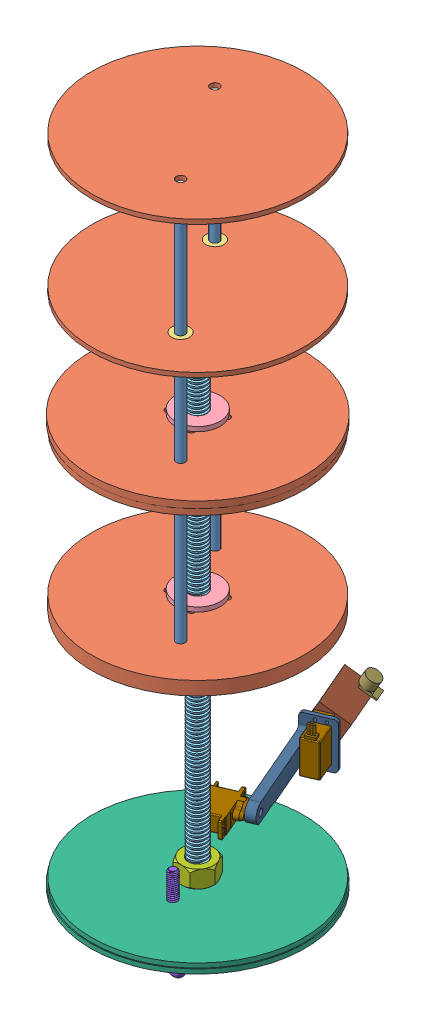
SolidWorks assembly Payload, configuration Default. Lengths in mm.
Overall size (210.78 503.44 275.7).
24 component instances, 15 part files, 42 mates.
Components (placement in the parent):
- Payload Bay-1: Payload Bay [Default] at (141.5956 144.8149 195.4526) size (155.24 279.4 155.24) (hidden)
- Payload Airframe-1: Payload Airframe [Default] at (141.5956 195.6149 195.4526) x (-0.336591 0 -0.941651) z (0.941651 0 -0.336591) size (155.24 254 155.24) (hidden)
- Nosecone-1: Nosecone [Default] at (141.5956 1055.8458 195.4526) x (0 -1 0) z (-0.561903 0 0.827203) size (742.76 155.24 155.24) (hidden)
- Steel Rod-1: Steel Rod [Default] at (119.1458 155.9274 160.8169) x (-0.543909 0 -0.839144) z (0.839144 0 -0.543909) size (6.35 288.93 6.35)
- Steel Rod-2: Steel Rod [Default] at (164.0455 155.9274 230.0882) x (-0.543909 0 -0.839144) z (0.839144 0 -0.543909) size (6.35 288.93 6.35)
- Central Mount-3: Central Mount [Motor Mount] at (141.5956 352.0501 195.4526) x (-0.543909 0 -0.839144) z (0.839144 0 -0.543909) size (150.98 3.17 150.98)
- 6389K627_Light Duty Dry-Running Nylon Sleeve Bearing-1: 6389K627_Light Duty Dry-Running Nylon Sleeve Bearing [6389K627] at (119.1458 355.2251 160.8169) x (0.493731 0 0.869615) z (0.869615 0 -0.493731) size (12.7 9.53 12.7)
- 6389K627_Light Duty Dry-Running Nylon Sleeve Bearing-2: 6389K627_Light Duty Dry-Running Nylon Sleeve Bearing [6389K627] at (164.0455 355.2251 230.0882) x (-0.837169 0 -0.546944) z (-0.546944 0 0.837169) size (12.7 9.53 12.7)
- Central Mount-4: Central Mount [Screw Mount Top] at (141.5956 276.5774 195.4526) x (-0.543909 0 -0.839144) z (-0.839144 0 0.543909) size (152.4 9.53 152.4)
- Central Mount-5: Central Mount [Copy of Screw Mount Bottom] at (141.5956 155.9274 195.4526) x (-0.543909 0 -0.839144) z (0.839144 0 -0.543909) size (150.98 9.53 150.98)
- Central Mount-6: Central Mount [Top Plate] at (141.5956 449.6149 195.4526) x (-0.543909 0 -0.839144) z (-0.839144 0 0.543909) size (150.98 3.17 150.98)
- 95120A111_932 Bearing Bronze Acme Flange Nut-1: 95120A111_932 Bearing Bronze Acme Flange Nut [95120A111] at (141.5956 279.7524 195.4526) x (0.056164 0 0.998422) z (0.998422 0 -0.056164) size (31.75 26.14 31.75)
- 95120A111_932 Bearing Bronze Acme Flange Nut-2: 95120A111_932 Bearing Bronze Acme Flange Nut [95120A111] at (141.5956 168.6274 195.4526) x (0.056164 0 0.998422) z (0.998422 0 -0.056164) size (31.75 26.14 31.75)
- 98935A911_Carbon Steel Acme Lead Screw-1: 98935A911_Carbon Steel Acme Lead Screw [98935A911] at (141.5956 47.2501 195.4526) x (0 1 0) z (-0.83707 0 0.547095) size (382.87 12.7 14.66)
- Bulkhead-1: Bulkhead [Default] at (141.5956 -14.9303 195.4526) x (0.918474 0 -0.395481) z (0.395481 0 0.918474) size (152.4 6.35 152.4)
- 94815A107_Carbon Steel Acme Hex Nut-1: 94815A107_Carbon Steel Acme Hex Nut [94815A107] at (141.5956 -21.0818 195.4526) x (0.073978 0 0.99726) z (0 1 0) size (22.23 28.23 12.35)
- 94815A107_Carbon Steel Acme Hex Nut-2: 94815A107_Carbon Steel Acme Hex Nut [94815A107] at (141.5956 -2.4287 195.4526) x (0.837169 0 0.546944) z (0 1 0) size (22.23 28.23 12.35)
- 3014T45_Steel Eyebolt with Shoulder - for Lifting-1: 3014T45_Steel Eyebolt with Shoulder - for Lifting [3014T45] at (147.1643 -38.7428 218.6369) x (-0.930118 0 -0.367262) z (-0.367262 0 0.930118) size (30.16 64.79 14.29)
- Gimbal Assem-1: Gimbal Assem [Default] at (112.6369 -2.8653 153.4838) x (0 -1 0) z (0.395481 0 0.918474) size (36.8 57.45 135.7) (flexible)
  - Hitec HS-65mg+ Micro Servo v01-1: Hitec HS-65mg+ Micro Servo v01 [Default] at origin size (11.43 28.88 36.23)
  - Camera Arm-1: Camera Arm [Default] at (0 18.675 -37.6301) size (32.79 21.59 76.2)
  - Hitec HS-65mg+ Micro Servo v01-2: Hitec HS-65mg+ Micro Servo v01 [Default] at (0 27.565 -68.0533) x (0 -1 0) z (1 0 0) size (11.43 28.88 36.23)
  - Camera Mount-1: Camera Mount [Default] at (-10.3181 30.0369 -83.5533) x (0.486593 0.873629 0) z (-0.873629 0.486593 0) size (20 35 12.7)
  - Arducam Camera-1: Arducam Camera [Default] at (-8.7661 38.0435 -114.3033) x (-0.486593 -0.873629 0) z (0 0 -1) size (13.5 9 10)
Mates (geometry in assembly coordinates):
- Concentric1: concentric aligned: circle of Payload Bay-1; circle of Payload Airframe-1
- Coincident2: coincident anti-aligned: plane of Payload Bay-1 through (141.5956 195.6149 195.4526) normal (0 1 0); plane of Payload Airframe-1 through (141.5956 195.6149 195.4526) normal (0 -1 0)
- Concentric3: concentric anti-aligned: cylinder of Payload Airframe-1 through (141.5956 449.6149 195.4526) axis (0 -1 0) radius 76.2; cylinder of Nosecone-1 through (141.5956 1055.8458 195.4526) axis (0 1 0) radius 76.2
- Coincident4: coincident anti-aligned: plane of Payload Airframe-1 through (141.5956 449.6149 195.4526) normal (0 1 0); plane of Nosecone-1 through (141.5956 449.6149 195.4526) normal (0 -1 0)
- Concentric6: concentric aligned: circle of Steel Rod-1; cylinder of Central Mount-3 through (119.1458 324.7451 160.8169) axis (0 1 0) radius 4.7625
- Concentric7: concentric anti-aligned: circle of Steel Rod-2; circle of Central Mount-3
- Concentric8: concentric anti-aligned: cylinder of Steel Rod-1 through (119.1458 444.8524 160.8169) axis (0 -1 0) radius 3.175; cylinder of 6389K627_Light Duty Dry-Running Nylon Sleeve Bearing-1 through (119.1458 345.7001 160.8169) axis (0 1 0) radius 3.175
- Coincident10: coincident anti-aligned: plane of Central Mount-3 through (119.1458 353.6376 160.8169) normal (0 1 0); plane of 6389K627_Light Duty Dry-Running Nylon Sleeve Bearing-1 through (119.1458 353.6376 160.8169) normal (0 -1 0)
- Concentric9: concentric anti-aligned: cylinder of Steel Rod-2 through (164.0455 444.8524 230.0882) axis (0 -1 0) radius 3.175; cylinder of 6389K627_Light Duty Dry-Running Nylon Sleeve Bearing-2 through (164.0455 345.7001 230.0882) axis (0 1 0) radius 4.7625
- Coincident11: coincident anti-aligned: plane of Central Mount-3 through (164.0455 353.6376 230.0882) normal (0 1 0); plane of 6389K627_Light Duty Dry-Running Nylon Sleeve Bearing-2 through (164.0455 353.6376 230.0882) normal (0 -1 0)
- Concentric10: concentric aligned: cylinder of Steel Rod-2 through (164.0455 444.8524 230.0882) axis (0 -1 0) radius 3.175; cylinder of Central Mount-4 through (164.0455 276.5774 230.0882) axis (0 -1 0) radius 3.175
- Coincident12: coincident aligned: cylinder of Steel Rod-1 through (119.1458 444.8524 160.8169) axis (0 -1 0) radius 3.175; circle of Central Mount-4
- Concentric11: concentric anti-aligned: cylinder of Steel Rod-2 through (164.0455 444.8524 230.0882) axis (0 -1 0) radius 3.175; cylinder of Central Mount-5 through (164.0455 160.6899 230.0882) axis (0 1 0) radius 3.175
- Concentric12: concentric anti-aligned: cylinder of Payload Bay-1 through (141.5956 -7.5851 195.4526) axis (0 1 0) radius 75.4888; cylinder of Central Mount-5 through (141.5956 165.4524 195.4526) axis (0 -1 0) radius 75.4888
- Coincident15: coincident anti-aligned: plane of Payload Bay-1 through (141.5956 271.8149 195.4526) normal (0 1 0); plane of Central Mount-4 through (141.5956 271.8149 195.4526) normal (0 -1 0)
- Distance1: distance = 101.6 mm anti-aligned: plane of Central Mount-4 through (141.5956 267.0524 195.4526) normal (0 -1 0); plane of Central Mount-5 through (141.5956 165.4524 195.4526) normal (0 1 0)
- Concentric13: concentric aligned: cylinder of Steel Rod-1 through (119.1458 444.8524 160.8169) axis (0 -1 0) radius 3.175; cylinder of Central Mount-6 through (119.1458 451.2024 160.8169) axis (0 -1 0) radius 3.175
- Concentric14: concentric aligned: cylinder of Steel Rod-2 through (164.0455 444.8524 230.0882) axis (0 -1 0) radius 3.175; cylinder of Central Mount-6 through (164.0455 451.2024 230.0882) axis (0 -1 0) radius 3.175
- Coincident17: coincident anti-aligned: circle of Steel Rod-1; circle of Central Mount-6
- Concentric15: concentric aligned: cylinder of Payload Bay-1 through (141.5956 -7.5851 195.4526) axis (0 1 0) radius 76.2; cylinder of Central Mount-4 through (141.5956 267.0524 195.4526) axis (0 1 0) radius 76.2
- Concentric17: concentric aligned: cylinder of Central Mount-4 through (141.5956 305.9144 195.4526) axis (0 -1 0) radius 9.525; cylinder of 95120A111_932 Bearing Bronze Acme Flange Nut-1 through (141.5956 325.1027 195.4526) axis (0 -1 0) radius 9.525
- Coincident19: coincident anti-aligned: plane of Central Mount-4 through (141.5956 276.5774 195.4526) normal (0 1 0); plane of 95120A111_932 Bearing Bronze Acme Flange Nut-1 through (141.5956 276.5774 195.4526) normal (0 -1 0)
- Concentric18: concentric anti-aligned: cylinder of Central Mount-5 through (141.5956 126.5904 195.4526) axis (0 1 0) radius 9.525; cylinder of 95120A111_932 Bearing Bronze Acme Flange Nut-2 through (141.5956 213.9777 195.4526) axis (0 -1 0) radius 9.525
- Coincident20: coincident anti-aligned: plane of Central Mount-5 through (141.5956 165.4524 195.4526) normal (0 1 0); plane of 95120A111_932 Bearing Bronze Acme Flange Nut-2 through (141.5956 165.4524 195.4526) normal (0 -1 0)
- Concentric19: concentric anti-aligned: circle of 95120A111_932 Bearing Bronze Acme Flange Nut-1; circle of 98935A911_Carbon Steel Acme Lead Screw-1
- Coincident21: coincident anti-aligned: plane of Central Mount-3 through (141.5956 352.0501 195.4526) normal (0 -1 0); plane of 98935A911_Carbon Steel Acme Lead Screw-1 through (141.5956 352.0501 195.4526) normal (0 1 0)
- Screw1: screw = 2.54 mm anti-aligned: cylinder of 95120A111_932 Bearing Bronze Acme Flange Nut-2 through (141.5956 168.6284 195.4526) axis (0 -1 0) radius 6.35; cylinder of 98935A911_Carbon Steel Acme Lead Screw-1 through (141.5956 -257.5499 195.4526) axis (0 1 0) radius 6.35
- LimitDistance1: limit distance = 75.4727 mm anti-aligned: plane of Central Mount-3 through (141.5956 352.0501 195.4526) normal (0 -1 0); plane of Central Mount-4 through (141.5956 276.5774 195.4526) normal (0 1 0)
- Coincident23: coincident aligned: plane of Steel Rod-1 through (119.1458 155.9274 160.8169) normal (0 -1 0); plane of Central Mount-5 through (141.5956 155.9274 195.4526) normal (0 -1 0)
- Coincident24: coincident aligned: plane of Steel Rod-2 through (164.0455 155.9274 230.0882) normal (0 -1 0); plane of Central Mount-5 through (141.5956 155.9274 195.4526) normal (0 -1 0)
- Concentric21: concentric aligned: circle of 98935A911_Carbon Steel Acme Lead Screw-1; circle of Bulkhead-1
- LimitDistance2: limit distance = 4.1701 mm anti-aligned: plane of Bulkhead-1 through (141.5956 -11.7553 195.4526) normal (0 1 0); plane of Payload Bay-1 through (141.5956 -7.5851 195.4526) normal (0 -1 0)
- Concentric23: concentric aligned: circle of 98935A911_Carbon Steel Acme Lead Screw-1; circle of 94815A107_Carbon Steel Acme Hex Nut-1
- Coincident31: coincident anti-aligned: plane of Bulkhead-1 through (141.5956 -14.9303 195.4526) normal (0 -1 0); plane of 94815A107_Carbon Steel Acme Hex Nut-1 through (128.7992 -14.9303 196.4018) normal (0 1 0)
- Distance7: distance = 14.0197 mm aligned: plane of Bulkhead-1 through (141.5956 -14.9303 195.4526) normal (0 -1 0); plane of 98935A911_Carbon Steel Acme Lead Screw-1 through (141.5956 -28.9499 195.4526) normal (0 -1 0)
- Concentric24: concentric aligned: circle of 98935A911_Carbon Steel Acme Lead Screw-1; circle of 94815A107_Carbon Steel Acme Hex Nut-2
- Coincident35: coincident anti-aligned: plane of Bulkhead-1 through (141.5956 -8.5803 195.4526) normal (0 1 0); plane of 94815A107_Carbon Steel Acme Hex Nut-2 through (134.5775 -8.5803 206.1948) normal (0 -1 0)
- Coincident36: coincident anti-aligned: plane of Bulkhead-1 through (141.5956 -14.9303 195.4526) normal (0 -1 0); plane of 3014T45_Steel Eyebolt with Shoulder - for Lifting-1 through (147.1643 -14.9303 218.6369) normal (0 1 0)
- Lock2: lock: unknown of Bulkhead-1; unknown of 3014T45_Steel Eyebolt with Shoulder - for Lifting-1
- Coincident37: coincident anti-aligned: plane of Bulkhead-1 through (141.5956 -8.5803 195.4526) normal (0 1 0); plane of Gimbal Assem-1/Hitec HS-65mg+ Micro Servo v01-1 through (108.1583 -8.5803 168.3683) normal (0 -1 0)
- Distance8: distance = 38.1 mm aligned: plane of Gimbal Assem-1/Hitec HS-65mg+ Micro Servo v01-1 through (126.5278 -8.5803 160.4587) normal (0.395481 0 0.918474); plane of Bulkhead-1 through (141.5956 -14.9303 195.4526) normal (0.395481 0 0.918474)
- Coincident40: coincident aligned: plane of Bulkhead-1 through (141.5956 -14.9303 195.4526) normal (0.918474 0 -0.395481); plane of Gimbal Assem-1/Hitec HS-65mg+ Micro Servo v01-1 through (126.5278 -8.5803 160.4587) normal (0.918474 0 -0.395481)
